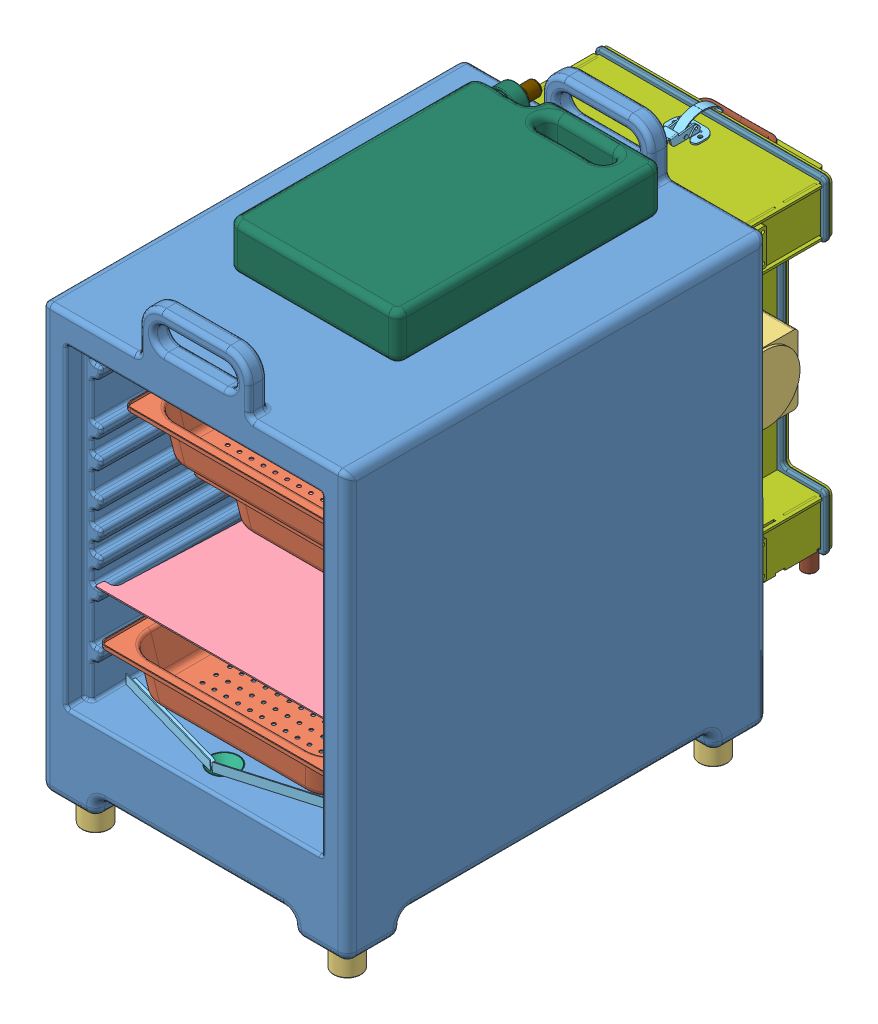
SolidWorks assembly FMT.201, configuration FULL ASSEMBLY. Lengths in mm.
Overall size (425.45 698.5 816.55).
103 component instances, 37 part files, 199 mates.
Components (placement in the parent):
- FMT.003-1: FMT.003 [Default] at origin size (425.45 660.4 584.2)
- FMT.004-1: FMT.004 [Default] at (0 188.9125 -205.3413) x (0 0 -1) z (1 0 0) size (352.43 61.91 323.85)
- FMT.004-2: FMT.004 [Default] at (0 457.2 -240.4686) x (0 0 -1) z (1 0 0) size (352.43 61.91 323.85)
- FMT.004-3: FMT.004 [Default] at (0 333.375 -332.9533) x (0 0 -1) z (1 0 0) size (352.43 61.91 323.85)
- 9540K743 Rubber Bumper with Unthreaded Hole-1: 9540K743 Rubber Bumper with Unthreaded Hole [Default] at (174.625 0 -546.1) x (-0.837169 0 -0.546944) z (-0.546944 0 0.837169) size (38.1 38.1 38.1)
- 9540K743 Rubber Bumper with Unthreaded Hole-2: 9540K743 Rubber Bumper with Unthreaded Hole [Default] at (-174.625 0 -546.1) x (-0.837169 0 -0.546944) z (-0.546944 0 0.837169) size (38.1 38.1 38.1)
- 9540K743 Rubber Bumper with Unthreaded Hole-3: 9540K743 Rubber Bumper with Unthreaded Hole [Default] at (174.625 0 -38.1) x (-0.837169 0 -0.546944) z (-0.546944 0 0.837169) size (38.1 38.1 38.1)
- 9540K743 Rubber Bumper with Unthreaded Hole-4: 9540K743 Rubber Bumper with Unthreaded Hole [Default] at (-174.625 0 -38.1) x (-0.837169 0 -0.546944) z (-0.546944 0 0.837169) size (38.1 38.1 38.1)
- FMT.008-1: FMT.008 [Default] at (0 524.3716 -59.6438) x (1 0 0) z (0 -0.039103 -0.999235) size (323.85 16 381)
- FMT.008-2: FMT.008 [Default] at (0 367.2091 -522.2121) x (-1 0 0) z (0 -0.039103 0.999235) size (323.85 16 381)
- FMT.008-3: FMT.008 [Default] at (0 257.7083 -24.2781) x (1 0 0) z (0 -0.041994 -0.999118) size (323.85 16 381)
- 1755K11 Clear Polycarbonate 90 Degree Angle-1: 1755K11 Clear Polycarbonate 90 Degree Angle [RIGHT] at (1.3565 116.5175 -24.0575) x (-0.267235 0.025225 -0.963301) z (0.963631 0.006995 -0.267144) size (12.7 12.7 171.45)
- 1755K11 Clear Polycarbonate 90 Degree Angle-2: 1755K11 Clear Polycarbonate 90 Degree Angle [LEFT] at (-166.5711 117.7168 -69.8593) x (0.267235 0.025225 -0.963301) z (0.963631 -0.006995 0.267144) size (12.7 12.7 171.45)
- 1479T83 Plastic Funnel-1: 1479T83 Plastic Funnel [Default] at (0 116.9717 -41.4022) x (1 0 0) z (0 -0.026177 0.999657) size (41.06 50.69 41.06)
- FMT.101-1: FMT.101 [Default] at (0 335.28 -596.6968) x (-1 0 0) z (0 0 -1) size (320.04 454.66 222.83)
- 9602K410_CORROSION-RESISTANT EQUIPMENT-COOLING FAN-1: 9602K410_CORROSION-RESISTANT EQUIPMENT-COOLING FAN [Default] at (-0.0145 289.8918 -660.2113) x (-1 0 0) z (0 -1 0) size (120 120 38)
- 92949A148_18-8 SS BUTTON-HEAD SOCKET CAP SCREW-1: 92949A148_18-8 SS BUTTON-HEAD SOCKET CAP SCREW [92949A148] at (52.4855 259.746 -712.7113) x (0.019534 0 -0.999809) z (0 1 0) size (6.65 6.65 14.96)
- 92949A148_18-8 SS BUTTON-HEAD SOCKET CAP SCREW-2: 92949A148_18-8 SS BUTTON-HEAD SOCKET CAP SCREW [92949A148] at (52.4855 259.746 -607.6823) x (0.019534 0 -0.999809) z (0 1 0) size (6.65 6.65 14.96)
- 92949A148_18-8 SS BUTTON-HEAD SOCKET CAP SCREW-3: 92949A148_18-8 SS BUTTON-HEAD SOCKET CAP SCREW [92949A148] at (-52.5435 259.746 -712.7113) x (0.019534 0 -0.999809) z (0 1 0) size (6.65 6.65 14.96)
- 92949A148_18-8 SS BUTTON-HEAD SOCKET CAP SCREW-4: 92949A148_18-8 SS BUTTON-HEAD SOCKET CAP SCREW [92949A148] at (-52.5435 259.746 -607.6823) x (0.019534 0 -0.999809) z (0 1 0) size (6.65 6.65 14.96)
- FMT.202-1: FMT.202 [Default] at (0 58.42 -584.2) x (-1 0 0) z (0 0 -1) size (304.8 50.8 24)
- 1661A100_LOAD-RATED PULL HANDLE WITH THREADED HOLES-1: 1661A100_LOAD-RATED PULL HANDLE WITH THREADED HOLES [1661A1] at (0 147.32 -726.6686) x (1 0 0) z (0 0 -1) size (120.8 23.9 38.64)
- 1661A100_LOAD-RATED PULL HANDLE WITH THREADED HOLES-2: 1661A100_LOAD-RATED PULL HANDLE WITH THREADED HOLES [1661A1] at (0 523.24 -726.6686) x (1 0 0) z (0 0 -1) size (120.8 23.9 38.64)
- 92949A537_18-8 SS BUTTON-HEAD SOCKET CAP SCREW-1: 92949A537_18-8 SS BUTTON-HEAD SOCKET CAP SCREW [92949A537] at (-52.3875 147.32 -720.344) x (0.730716 0.682681 0) z (0 0 1) size (11.1 11.1 16.71)
- 92949A537_18-8 SS BUTTON-HEAD SOCKET CAP SCREW-2: 92949A537_18-8 SS BUTTON-HEAD SOCKET CAP SCREW [92949A537] at (52.3875 147.32 -720.344) x (0.730716 0.682681 0) z (0 0 1) size (11.1 11.1 16.71)
- 92949A537_18-8 SS BUTTON-HEAD SOCKET CAP SCREW-3: 92949A537_18-8 SS BUTTON-HEAD SOCKET CAP SCREW [92949A537] at (-52.3875 523.24 -720.344) x (0.730716 0.682681 0) z (0 0 1) size (11.1 11.1 16.71)
- 92949A537_18-8 SS BUTTON-HEAD SOCKET CAP SCREW-4: 92949A537_18-8 SS BUTTON-HEAD SOCKET CAP SCREW [92949A537] at (52.3875 523.24 -720.344) x (0.730716 0.682681 0) z (0 0 1) size (11.1 11.1 16.71)
- 91830A101_18-8 STAINLESS STEEL KNURLED HEAD THUMB SCREW-1: 91830A101_18-8 STAINLESS STEEL KNURLED HEAD THUMB SCREW [91830A101] at (142.875 523.24 -726.6686) x (-0.923728 -0.383049 0) z (0 0 -1) size (9.52 9.52 12.12)
- 91830A101_18-8 STAINLESS STEEL KNURLED HEAD THUMB SCREW-2: 91830A101_18-8 STAINLESS STEEL KNURLED HEAD THUMB SCREW [91830A101] at (-142.875 523.24 -726.6686) x (-0.923728 -0.383049 0) z (0 0 -1) size (9.52 9.52 12.12)
- 91830A101_18-8 STAINLESS STEEL KNURLED HEAD THUMB SCREW-3: 91830A101_18-8 STAINLESS STEEL KNURLED HEAD THUMB SCREW [91830A101] at (142.875 147.32 -726.6686) x (-0.923728 0.383049 0) z (0 0 -1) size (9.52 9.52 12.12)
- 91830A101_18-8 STAINLESS STEEL KNURLED HEAD THUMB SCREW-4: 91830A101_18-8 STAINLESS STEEL KNURLED HEAD THUMB SCREW [91830A101] at (-142.875 147.32 -726.6686) x (-0.923728 0.383049 0) z (0 0 -1) size (9.52 9.52 12.12)
- 91830A101_18-8 STAINLESS STEEL KNURLED HEAD THUMB SCREW-5: 91830A101_18-8 STAINLESS STEEL KNURLED HEAD THUMB SCREW [91830A101] at (85.725 436.88 -726.6686) x (-0.923728 -0.383049 0) z (0 0 -1) size (9.52 9.52 12.12)
- 91780A560_ALUM FEM THRDED HEX STANDOFF-1: 91780A560_ALUM FEM THRDED HEX STANDOFF [91780A560] at (142.875 523.24 -660.1968) size (6.35 7.33 127.86)
- 91780A560_ALUM FEM THRDED HEX STANDOFF-4: 91780A560_ALUM FEM THRDED HEX STANDOFF [91780A560] at (142.875 147.32 -660.1968) size (6.35 7.33 127.86)
- 91780A560_ALUM FEM THRDED HEX STANDOFF-2: 91780A560_ALUM FEM THRDED HEX STANDOFF [91780A560] at (-142.875 523.24 -660.1968) size (6.35 7.33 127.86)
- 91780A560_ALUM FEM THRDED HEX STANDOFF-3: 91780A560_ALUM FEM THRDED HEX STANDOFF [91780A560] at (-142.875 147.32 -660.1968) size (6.35 7.33 127.86)
- 91780A560_ALUM FEM THRDED HEX STANDOFF-5: 91780A560_ALUM FEM THRDED HEX STANDOFF [91780A560] at (85.725 436.88 -660.1968) size (6.35 7.33 127.86)
- 91780A560_ALUM FEM THRDED HEX STANDOFF-6: 91780A560_ALUM FEM THRDED HEX STANDOFF [91780A560] at (-85.725 436.88 -660.1968) size (6.35 7.33 127.86)
- 91830A101_18-8 STAINLESS STEEL KNURLED HEAD THUMB SCREW-6: 91830A101_18-8 STAINLESS STEEL KNURLED HEAD THUMB SCREW [91830A101] at (-85.725 436.88 -726.6686) x (-0.923728 -0.383049 0) z (0 0 -1) size (9.52 9.52 12.12)
- Heating Element-1: Heating Element [Default] at (-2.4765 289.8918 -660.3873) x (0 0 1) z (0 1 0) size (119.38 122.68 24.13)
- 91830A101_18-8 STAINLESS STEEL KNURLED HEAD THUMB SCREW-7: 91830A101_18-8 STAINLESS STEEL KNURLED HEAD THUMB SCREW [91830A101] at (85.725 233.68 -726.6686) x (-0.923728 0.383049 0) z (0 0 -1) size (9.52 9.52 12.12)
- 91830A101_18-8 STAINLESS STEEL KNURLED HEAD THUMB SCREW-8: 91830A101_18-8 STAINLESS STEEL KNURLED HEAD THUMB SCREW [91830A101] at (-85.725 233.68 -726.6686) x (-0.923728 0.383049 0) z (0 0 -1) size (9.52 9.52 12.12)
- 91780A560_ALUM FEM THRDED HEX STANDOFF-7: 91780A560_ALUM FEM THRDED HEX STANDOFF [91780A560] at (-85.725 233.68 -660.1968) size (6.35 7.33 127.86)
- 91780A560_ALUM FEM THRDED HEX STANDOFF-8: 91780A560_ALUM FEM THRDED HEX STANDOFF [91780A560] at (85.725 233.68 -660.1968) size (6.35 7.33 127.86)
- 4946A100_EXPANDABLE LOCKING GROMMETS-1: 4946A100_EXPANDABLE LOCKING GROMMETS [4946A1] at (-92.5512 283.6418 -660.1968) x (0 0.984877 -0.173256) z (0 -0.173256 -0.984877) size (16.67 6.35 16.67)
- 4946A100_EXPANDABLE LOCKING GROMMETS-2: 4946A100_EXPANDABLE LOCKING GROMMETS [4946A1] at (-92.5512 309.0418 -660.1968) x (0 -1 0) z (0 0 1) size (16.67 6.35 16.67)
- MCM 4629T35-1: MCM 4629T35 [Default] at (-57.15 50.8 -318.135) x (0 0 -1) z (-1 0 0) size (330.2 66.71 213.41)
- 1601N123-1: 1601N123 [Default] at (0 523.24 -593.725) size (304.8 76.2 9.53)
- 1601N123-2: 1601N123 [Default] at (0 147.32 -593.725) size (304.8 76.2 9.53)
- MCM 1659A7-1: MCM 1659A7 [FEMALE] at (-166.6875 523.24 -608.1268) x (0 1 0) z (0 0 1) size (46.61 12.7 31.75)
- MCM 1659A7-2: MCM 1659A7 [MALE] at (-168.5925 523.24 -622.3) x (0 1 0) z (0 0 1) size (46.61 12.7 31.75)
- FMT.203-2: FMT.203 [Default] at (-153.3525 711.581 -744.22) x (0 0 -1) z (-1 0 0) size (6.35 50.8 38.1)
- FMT.203-3: FMT.203 [Default] at (-153.3525 335.661 -744.22) x (0 0 -1) z (-1 0 0) size (6.35 50.8 38.1)
- MCM 1659A7-3: MCM 1659A7 [MALE] at (-168.5925 147.32 -622.3) x (0 1 0) z (0 0 1) size (46.61 12.7 31.75)
- MCM 1659A7-4: MCM 1659A7 [FEMALE] at (-166.6875 147.32 -608.1268) x (0 1 0) z (0 0 1) size (46.61 12.7 31.75)
- MCM 1659A7-5: MCM 1659A7 [MALE] at (168.5925 523.24 -622.3) x (0 -1 0) z (0 0 1) size (46.61 12.7 31.75)
- MCM 1659A7-6: MCM 1659A7 [FEMALE] at (166.6875 523.24 -608.1268) x (0 -1 0) z (0 0 1) size (46.61 12.7 31.75)
- MCM 1659A7-7: MCM 1659A7 [MALE] at (168.5925 147.32 -622.3) x (0 -1 0) z (0 0 1) size (46.61 12.7 31.75)
- MCM 1659A7-8: MCM 1659A7 [FEMALE] at (166.6875 147.32 -608.1268) x (0 -1 0) z (0 0 1) size (46.61 12.7 31.75)
- GeekTeches Thermoelectric Peltier Refrigeration Cooling System, Radiator Semiconductor Cooler Conduction Module Fan-1: GeekTeches Thermoelectric Peltier Refrigeration Cooling System, Radiator Semiconductor Cooler Conduction Module Fan [Default] at (144.145 339.5218 -646.2268) x (0 0 1) z (-1 0 0) size (96.52 96.52 96.52)
- FMT.011-1: FMT.011 [simplified mesh] at (0 477.3418 -686.4169) size (154.94 103.94 79.25)
- FMT.203-4: FMT.203 [Default] at (153.4556 335.661 -744.22) x (0 0 -1) z (1 0 0) size (6.35 50.8 38.1)
- FMT.203-5: FMT.203 [Default] at (153.4556 -40.259 -744.22) x (0 0 -1) z (1 0 0) size (6.35 50.8 38.1)
- 4946A100_EXPANDABLE LOCKING GROMMETS-3: 4946A100_EXPANDABLE LOCKING GROMMETS [4946A1] at (92.5512 283.6418 -660.1968) x (0 0 1) z (0 -1 0) size (16.67 6.35 16.67)
- 1863A210_DRAW LATCH-1: 1863A210_DRAW LATCH [Default] at (-0.0131 114.3 -684.9132) x (1 0 0) z (0 0 -1) size (47.62 20.89 96.69)
- 91115A834_18-8 SS FEM THRDED HEX STANDOFF-1: 91115A834_18-8 SS FEM THRDED HEX STANDOFF [91115A834] at (63.5 372.77 -685.5968) x (0.866025 -0.5 0) z (0 0 1) size (6.35 7.33 77.29)
- 92949A148_18-8 SS BUTTON-HEAD SOCKET CAP SCREW-5: 92949A148_18-8 SS BUTTON-HEAD SOCKET CAP SCREW [92949A148] at (63.5 372.77 -728.5228) x (-0.40102 0.916069 0) z (0 0 -1) size (6.65 6.65 14.96)
- 91115A834_18-8 SS FEM THRDED HEX STANDOFF-2: 91115A834_18-8 SS FEM THRDED HEX STANDOFF [91115A834] at (-63.5 372.77 -685.5968) x (0.866025 -0.5 0) z (0 0 1) size (6.35 7.33 77.29)
- 91115A834_18-8 SS FEM THRDED HEX STANDOFF-3: 91115A834_18-8 SS FEM THRDED HEX STANDOFF [91115A834] at (0 372.77 -685.5968) x (0 -1 0) z (0 0 1) size (6.35 7.33 77.29)
- 92949A148_18-8 SS BUTTON-HEAD SOCKET CAP SCREW-6: 92949A148_18-8 SS BUTTON-HEAD SOCKET CAP SCREW [92949A148] at (0 372.77 -728.5228) x (-0.40102 0.916069 0) z (0 0 -1) size (6.65 6.65 14.96)
- 92949A148_18-8 SS BUTTON-HEAD SOCKET CAP SCREW-7: 92949A148_18-8 SS BUTTON-HEAD SOCKET CAP SCREW [92949A148] at (-63.5 372.77 -728.5228) x (0.270829 0.962628 0) z (0 0 -1) size (6.65 6.65 14.96)
- FMT.204-1: FMT.204 [Default] at (0.7958 326.6119 -867.9228) size (152.7 2.97 76.7)
- FITNATE Mist Maker-1: FITNATE Mist Maker [Default] at (0.0034 328.1168 -786.3887) size (44.45 42.67 44.45)
- FITNATE Mist Maker-2: FITNATE Mist Maker [Default] at (57.1534 328.1168 -786.3887) size (44.45 42.67 44.45)
- FMT.205-1: FMT.205 [Default] at (-0.7958 313.9119 -504.9109) x (-1 0 0) z (0 0 -1) size (130 6.35 60)
- 91115A135_18-8 SS FEM THRDED HEX STANDOFF-1: 91115A135_18-8 SS FEM THRDED HEX STANDOFF [91115A135] at (50 439.1338 -686.4169) x (1 0 0) z (0 1 0) size (6.35 7.33 39.19)
- 91115A135_18-8 SS FEM THRDED HEX STANDOFF-2: 91115A135_18-8 SS FEM THRDED HEX STANDOFF [91115A135] at (-50 439.1338 -686.4169) x (1 0 0) z (0 1 0) size (6.35 7.33 39.19)
- 1661A100_LOAD-RATED PULL HANDLE WITH THREADED HOLES-3: 1661A100_LOAD-RATED PULL HANDLE WITH THREADED HOLES [1661A1] at (0 441.3418 -726.0409) x (1 0 0) z (0 0 -1) size (120.8 23.9 38.64)
- 92949A537_18-8 SS BUTTON-HEAD SOCKET CAP SCREW-5: 92949A537_18-8 SS BUTTON-HEAD SOCKET CAP SCREW [92949A537] at (-52.3875 441.3418 -721.4181) x (0.730716 0.682681 0) z (0 0 1) size (11.1 11.1 16.71)
- 92949A537_18-8 SS BUTTON-HEAD SOCKET CAP SCREW-6: 92949A537_18-8 SS BUTTON-HEAD SOCKET CAP SCREW [92949A537] at (52.3875 441.3418 -721.4181) x (0.730716 0.682681 0) z (0 0 1) size (11.1 11.1 16.71)
- 1863A210_DRAW LATCH-2: 1863A210_DRAW LATCH [Default] at (0.0131 556.26 -684.9132) x (-1 0 0) z (0 0 -1) size (47.62 20.89 96.69)
- 9540K731 Rubber Bumper with Unthreaded Hole-1: 9540K731 Rubber Bumper with Unthreaded Hole [Default] at (142.875 114.3 -710.9968) x (-0.837169 0 -0.546944) z (-0.546944 0 0.837169) size (19.05 25.4 19.05)
- 9540K731 Rubber Bumper with Unthreaded Hole-2: 9540K731 Rubber Bumper with Unthreaded Hole [Default] at (-142.875 114.3 -710.9968) x (-0.837169 0 -0.546944) z (-0.546944 0 0.837169) size (19.05 25.4 19.05)
- 9540K731 Rubber Bumper with Unthreaded Hole-3: 9540K731 Rubber Bumper with Unthreaded Hole [Default] at (142.875 114.3 -619.125) x (-0.837169 0 -0.546944) z (-0.546944 0 0.837169) size (19.05 25.4 19.05)
- 9540K731 Rubber Bumper with Unthreaded Hole-4: 9540K731 Rubber Bumper with Unthreaded Hole [Default] at (-142.875 114.3 -619.125) x (-0.826006 0 -0.563662) z (-0.563662 0 0.826006) size (19.05 25.4 19.05)
- 92949A153_18-8 SS BUTTON-HEAD SOCKET CAP SCREW-1: 92949A153_18-8 SS BUTTON-HEAD SOCKET CAP SCREW [92949A153] at (-142.875 93.3958 -710.9968) x (-0.837051 0 -0.547124) z (0 -1 0) size (6.65 6.65 27.74)
- 92949A153_18-8 SS BUTTON-HEAD SOCKET CAP SCREW-2: 92949A153_18-8 SS BUTTON-HEAD SOCKET CAP SCREW [92949A153] at (-142.875 93.3958 -619.125) x (-0.837169 0 -0.546944) z (0 -1 0) size (6.65 6.65 27.74)
- 92949A153_18-8 SS BUTTON-HEAD SOCKET CAP SCREW-3: 92949A153_18-8 SS BUTTON-HEAD SOCKET CAP SCREW [92949A153] at (142.875 93.3958 -619.125) x (-0.837169 0 -0.546944) z (0 -1 0) size (6.65 6.65 27.74)
- 92949A153_18-8 SS BUTTON-HEAD SOCKET CAP SCREW-4: 92949A153_18-8 SS BUTTON-HEAD SOCKET CAP SCREW [92949A153] at (142.875 93.3958 -710.9968) x (-0.837169 0 -0.546944) z (0 -1 0) size (6.65 6.65 27.74)
- 91841A007_TYPE 18-8 STAINLESS STEEL HEX NUT-1: 91841A007_TYPE 18-8 STAINLESS STEEL HEX NUT [91841A007] at (-142.875 118.6609 -710.9968) size (7.94 3.39 9.17)
- 91841A007_TYPE 18-8 STAINLESS STEEL HEX NUT-2: 91841A007_TYPE 18-8 STAINLESS STEEL HEX NUT [91841A007] at (142.875 118.6609 -619.125) size (7.94 3.39 9.17)
- 91841A007_TYPE 18-8 STAINLESS STEEL HEX NUT-3: 91841A007_TYPE 18-8 STAINLESS STEEL HEX NUT [91841A007] at (142.875 118.6609 -710.9968) size (7.94 3.39 9.17)
- 91841A007_TYPE 18-8 STAINLESS STEEL HEX NUT-4: 91841A007_TYPE 18-8 STAINLESS STEEL HEX NUT [91841A007] at (-142.875 118.6609 -619.125) size (7.94 3.39 9.17)
- 93085K11 Surface-Mount, Hollow, 375 Wide, 1875 ID Rubber Seal-1: 93085K11 Surface-Mount, Hollow, 375 Wide, 1875 ID Rubber Seal [Default] at (0 335.28 -843.0768) size (320.04 454.66 7.62)
- 1542N2 HDPE TANK-1: 1542N2 HDPE TANK [Default] at (0 590.55 -349.25) size (235.88 63.5 373.38)
- 5779K162_PUSH-TO-CONNECT TUBE FITTING FOR AIR-1: 5779K162_PUSH-TO-CONNECT TUBE FITTING FOR AIR [5779K162] at (-59.47 465.3418 -734.9766) x (-1 0 0) z (0 0 -1) size (22.1 46.6 41.62)
- 5779K455_PUSH-TO-CONNECT TUBE FITTING FOR AIR-1: 5779K455_PUSH-TO-CONNECT TUBE FITTING FOR AIR [5779K455] at (-59.47 465.3418 -726.0409) x (-0.866025 -0.5 0) z (0 0 1) size (22.1 46.53 45.42)
- 5779K119_PUSH-TO-CONNECT TUBE FITTING FOR AIR-1: 5779K119_PUSH-TO-CONNECT TUBE FITTING FOR AIR [5779K119] at (-92.075 622.3 -528.2743) x (-0.079078 -0.996868 0) z (0 0 1) size (22 25.4 38.57)
- 50785K142_MED-PRESSURE BRASS THREADED PIPE FITTING-1: 50785K142_MED-PRESSURE BRASS THREADED PIPE FITTING [50785K142] at (-92.075 622.3 -533.4) x (0.619078 -0.78533 0) z (0 0 1) size (22.23 25.66 5.49)
- 92949A148_18-8 SS BUTTON-HEAD SOCKET CAP SCREW-8: 92949A148_18-8 SS BUTTON-HEAD SOCKET CAP SCREW [92949A148] at (50 466.3881 -686.4169) x (1 0 0) z (0 1 0) size (6.65 6.65 14.96)
- 92949A148_18-8 SS BUTTON-HEAD SOCKET CAP SCREW-9: 92949A148_18-8 SS BUTTON-HEAD SOCKET CAP SCREW [92949A148] at (-50 466.3881 -686.4169) x (1 0 0) z (0 1 0) size (6.65 6.65 14.96)
- 92949A148_18-8 SS BUTTON-HEAD SOCKET CAP SCREW-10: 92949A148_18-8 SS BUTTON-HEAD SOCKET CAP SCREW [92949A148] at (50 415.2578 -686.4169) x (-0.837169 0 -0.546944) z (0 -1 0) size (6.65 6.65 14.96)
- 92949A148_18-8 SS BUTTON-HEAD SOCKET CAP SCREW-11: 92949A148_18-8 SS BUTTON-HEAD SOCKET CAP SCREW [92949A148] at (-50 415.2578 -686.4169) x (-0.837169 0 -0.546944) z (0 -1 0) size (6.65 6.65 14.96)
Mates (geometry in assembly coordinates):
- Coincident1: coincident: plane of FMT.003-1 through (-212.725 0 -584.2) normal (0 -1 0); plane of assembly through (0 0 0) normal (0 1 0)
- Coincident2: coincident: plane of FMT.003-1 through (0 0 0) normal (1 0 0); plane of assembly through (0 0 0) normal (1 0 0)
- Coincident3: coincident: plane of FMT.003-1 through (0 0 0) normal (0 0 1); plane of assembly through (0 0 0) normal (0 0 1)
- Width4: width: plane of FMT.004-1 through (161.925 184.15 -29.1288) normal (1 0 0); plane of FMT.004-1 through (-161.925 184.15 -29.1288) normal (-1 0 0); plane of FMT.003-1 through (-167.4812 0 -25.4) normal (0.999962 0 0.008727); plane of FMT.003-1 through (167.4812 0 -25.4) normal (-0.999962 0 0.008727)
- Width5: width: plane of FMT.004-2 through (-161.925 452.4375 -64.2561) normal (-1 0 0); plane of FMT.004-2 through (161.925 452.4375 -64.2561) normal (1 0 0); plane of FMT.003-1 through (-167.4812 0 -25.4) normal (0.999962 0 0.008727); plane of FMT.003-1 through (167.4812 0 -25.4) normal (-0.999962 0 0.008727)
- Width6: width: plane of FMT.004-3 through (-161.925 328.6125 -156.7408) normal (-1 0 0); plane of FMT.004-3 through (161.925 328.6125 -156.7408) normal (1 0 0); plane of FMT.003-1 through (-167.4812 0 -25.4) normal (0.999962 0 0.008727); plane of FMT.003-1 through (167.4812 0 -25.4) normal (-0.999962 0 0.008727)
- Coincident12: coincident: plane of FMT.003-1 through (-167.4812 184.15 -572.1703) normal (0 1 0); plane of FMT.004-1 through (0 184.15 -205.3413) normal (0 -1 0)
- Coincident13: coincident: plane of FMT.003-1 through (-154.7812 328.6125 -572.1703) normal (0 1 0); plane of FMT.004-3 through (0 328.6125 -332.9533) normal (0 -1 0)
- Coincident14: coincident: plane of FMT.003-1 through (-167.4812 452.4375 -572.1703) normal (0 1 0); plane of FMT.004-2 through (0 452.4375 -240.4686) normal (0 -1 0)
- Coincident34: coincident: plane of FMT.003-1 through (-212.725 0 -584.2) normal (0 -1 0); plane of 9540K743 Rubber Bumper with Unthreaded Hole-1 through (174.625 0 -546.1) normal (0 1 0)
- Concentric4: concentric: cylinder of FMT.003-1 through (174.625 12.7 -546.1) axis (0 -1 0) radius 1.5875; cylinder of 9540K743 Rubber Bumper with Unthreaded Hole-1 through (174.625 -31.75 -546.1) axis (0 -1 0) radius 6.35
- Coincident35: coincident: plane of FMT.003-1 through (-212.725 0 -584.2) normal (0 -1 0); plane of 9540K743 Rubber Bumper with Unthreaded Hole-2 through (-174.625 0 -546.1) normal (0 1 0)
- Coincident36: coincident: plane of FMT.003-1 through (-212.725 0 -584.2) normal (0 -1 0); plane of 9540K743 Rubber Bumper with Unthreaded Hole-3 through (174.625 0 -38.1) normal (0 1 0)
- Coincident37: coincident: plane of FMT.003-1 through (-212.725 0 -584.2) normal (0 -1 0); plane of 9540K743 Rubber Bumper with Unthreaded Hole-4 through (-174.625 0 -38.1) normal (0 1 0)
- Concentric5: concentric: cylinder of FMT.003-1 through (-174.625 12.7 -546.1) axis (0 -1 0) radius 1.5875; cylinder of 9540K743 Rubber Bumper with Unthreaded Hole-2 through (-174.625 -38.1 -546.1) axis (0 1 0) radius 19.05
- Concentric6: concentric: cylinder of FMT.003-1 through (174.625 12.7 -38.1) axis (0 -1 0) radius 1.5875; cylinder of 9540K743 Rubber Bumper with Unthreaded Hole-3 through (174.625 -38.1 -38.1) axis (0 1 0) radius 19.05
- Concentric7: concentric: cylinder of FMT.003-1 through (-174.625 12.7 -38.1) axis (0 -1 0) radius 1.5875; cylinder of 9540K743 Rubber Bumper with Unthreaded Hole-4 through (-174.625 -38.1 -38.1) axis (0 1 0) radius 19.05
- Width17: width: plane of FMT.008-1 through (-146.05 518.7571 -243.715) normal (-1 0 0); plane of FMT.008-1 through (146.05 517.1709 -243.653) normal (1 0 0); plane of FMT.003-1 through (-212.725 590.55 -584.2) normal (-1 0 0); plane of FMT.003-1 through (212.725 590.55 -584.2) normal (1 0 0)
- Coincident43: coincident: plane of FMT.003-1 through (-167.4812 523.875 -572.1703) normal (0 1 0); line of FMT.008-1 through (-158.75 523.875 -72.3341) axis (1 0 0)
- Coincident44: coincident: plane of FMT.003-1 through (-167.4812 523.875 -572.1703) normal (0 1 0); line of FMT.008-1 through (-153.3525 523.875 -440.916) axis (-1 0 0)
- Width18: width: plane of FMT.008-2 through (-146.05 360.0084 -338.2029) normal (-1 0 0); plane of FMT.008-2 through (146.05 361.5946 -338.1409) normal (1 0 0); plane of FMT.003-1 through (212.725 590.55 -584.2) normal (1 0 0); plane of FMT.003-1 through (-212.725 590.55 -584.2) normal (-1 0 0)
- Coincident46: coincident: plane of FMT.003-1 through (-167.4812 366.7125 -572.1703) normal (0 1 0); line of FMT.008-2 through (-158.75 366.7125 -140.9399) axis (1 0 0)
- Coincident47: coincident: plane of FMT.003-1 through (-167.4812 366.7125 -572.1703) normal (0 1 0); line of FMT.008-2 through (-154.05 366.7125 -509.5218) axis (-1 0 0)
- Width19: width: plane of FMT.008-3 through (-146.05 251.5612 -208.3324) normal (-1 0 0); plane of FMT.008-3 through (146.05 249.9751 -208.2657) normal (1 0 0); plane of FMT.003-1 through (212.725 590.55 -584.2) normal (1 0 0); plane of FMT.003-1 through (-212.725 590.55 -584.2) normal (-1 0 0)
- Coincident48: coincident: plane of FMT.003-1 through (-154.7812 257.175 -572.1703) normal (0 1 0); line of FMT.008-3 through (-158.75 257.175 -380.1697) axis (1 0 0)
- Coincident49: coincident: plane of FMT.003-1 through (-154.7812 257.175 -572.1703) normal (0 1 0); line of FMT.008-3 through (-158.75 257.175 -36.9669) axis (1 0 0)
- Coincident52: coincident: plane of FMT.003-1 through (-167.4812 115.8875 0) normal (0 0.999657 0.026177); plane of 1755K11 Clear Polycarbonate 90 Degree Angle-1 through (163.1772 118.0372 -82.0932) normal (0 -0.999657 -0.026177)
- Parallel12: parallel: plane of FMT.003-1 through (167.4812 0 -25.4) normal (-0.999962 0 0.008727); line of 1755K11 Clear Polycarbonate 90 Degree Angle-1 through (163.2804 118.997 -70.2313) axis (-0.008724 0.026176 -0.999619)
- Coincident54: coincident: plane of FMT.003-1 through (-167.4812 115.8875 0) normal (0 0.999657 0.026177); plane of 1755K11 Clear Polycarbonate 90 Degree Angle-2 through (2.0374 116.8378 -36.2914) normal (0 -0.999657 -0.026177)
- Parallel13: parallel: plane of FMT.003-1 through (-167.4812 0 -25.4) normal (0.999962 0 0.008727); line of 1755K11 Clear Polycarbonate 90 Degree Angle-2 through (-163.1772 119.3068 -82.06) axis (-0.008724 -0.026176 0.999619)
- Width20: width: plane of 1755K11 Clear Polycarbonate 90 Degree Angle-1 through (1.3565 116.5175 -24.0575) normal (-0.870354 0.01289 -0.492257); plane of 1755K11 Clear Polycarbonate 90 Degree Angle-2 through (-1.3565 116.5175 -24.0575) normal (0.870354 0.01289 -0.492257); plane of FMT.003-1 through (212.725 590.55 -584.2) normal (1 0 0); plane of FMT.003-1 through (-212.725 590.55 -584.2) normal (-1 0 0)
- Coincident55: coincident: line of FMT.003-1 through (-159.1326 130.1736 -545.5647) axis (-0.008724 -0.026176 0.999619); point of 1755K11 Clear Polycarbonate 90 Degree Angle-2
- Coincident56: coincident: line of FMT.003-1 through (163.6384 116.6533 -29.2432) axis (-0.008724 0.026176 -0.999619); point of 1755K11 Clear Polycarbonate 90 Degree Angle-1
- Coincident65: coincident: plane of FMT.003-1 through (-167.4812 115.8875 0) normal (0 0.999657 0.026177); circle of 1479T83 Plastic Funnel-1
- Concentric11: concentric: cylinder of FMT.003-1 through (0 -14.1238 -44.8351) axis (0 0.999657 0.026177) radius 20.6375; cylinder of 1479T83 Plastic Funnel-1 through (0 116.9717 -41.4022) axis (0 0.999657 0.026177) radius 2.9527
- Coincident69: coincident: plane of 92949A537_18-8 SS BUTTON-HEAD SOCKET CAP SCREW-3 through (-48.5987 519.1846 -723.6968) normal (0 0 -1); plane of 92949A537_18-8 SS BUTTON-HEAD SOCKET CAP SCREW-4 through (56.1763 519.1846 -723.6968) normal (0 0 -1)
- Coincident70: coincident: plane of 92949A537_18-8 SS BUTTON-HEAD SOCKET CAP SCREW-2 through (56.1763 143.2646 -723.6968) normal (0 0 -1); plane of 92949A537_18-8 SS BUTTON-HEAD SOCKET CAP SCREW-4 through (56.1763 519.1846 -723.6968) normal (0 0 -1)
- Coincident71: coincident: plane of 92949A537_18-8 SS BUTTON-HEAD SOCKET CAP SCREW-1 through (-48.5987 143.2646 -723.6968) normal (0 0 -1); plane of 92949A537_18-8 SS BUTTON-HEAD SOCKET CAP SCREW-2 through (56.1763 143.2646 -723.6968) normal (0 0 -1)
- Distance8: distance = 9.525 mm: plane of FMT.003-1 through (0 0 -584.2) normal (0 0 -1); plane of FMT.101-1 through (0 335.28 -593.725) normal (0 0 1)
- Width32: width: plane of FMT.101-1 through (-153.67 335.28 -596.6968) normal (-1 0 0); plane of FMT.101-1 through (153.67 335.28 -596.6968) normal (1 0 0); plane of FMT.003-1 through (212.725 590.55 -584.2) normal (1 0 0); plane of FMT.003-1 through (-212.725 590.55 -584.2) normal (-1 0 0)
- Coincident96: coincident: plane of 92949A537_18-8 SS BUTTON-HEAD SOCKET CAP SCREW-1 through (-48.5987 143.2646 -723.6968) normal (0 0 -1); plane of FMT.101-1 through (-151.13 553.72 -723.6968) normal (0 0 1)
- Concentric24: concentric: circle of 92949A537_18-8 SS BUTTON-HEAD SOCKET CAP SCREW-3; circle of 1661A100_LOAD-RATED PULL HANDLE WITH THREADED HOLES-2
- Concentric25: concentric: circle of 1661A100_LOAD-RATED PULL HANDLE WITH THREADED HOLES-2; cylinder of FMT.101-1 through (-52.3875 523.24 -726.6686) axis (0 0 1) radius 3.175
- Concentric26: concentric: circle of 92949A537_18-8 SS BUTTON-HEAD SOCKET CAP SCREW-4; cylinder of FMT.101-1 through (52.3875 523.24 -726.6686) axis (0 0 1) radius 3.175
- Concentric27: concentric: circle of 92949A537_18-8 SS BUTTON-HEAD SOCKET CAP SCREW-4; circle of 1661A100_LOAD-RATED PULL HANDLE WITH THREADED HOLES-2
- Coincident98: coincident: plane of 1661A100_LOAD-RATED PULL HANDLE WITH THREADED HOLES-2 through (-46.0375 512.9212 -726.6686) normal (0 0 1); plane of FMT.101-1 through (-151.13 553.72 -726.6686) normal (0 0 -1)
- Concentric28: concentric: cylinder of 92949A537_18-8 SS BUTTON-HEAD SOCKET CAP SCREW-1 through (-52.3875 147.32 -720.344) axis (0 0 1) radius 5.5499; circle of FMT.101-1
- Concentric29: concentric: circle of 92949A537_18-8 SS BUTTON-HEAD SOCKET CAP SCREW-2; circle of FMT.101-1
- Coincident99: coincident: plane of 1661A100_LOAD-RATED PULL HANDLE WITH THREADED HOLES-1 through (46.0375 137.0012 -726.6686) normal (0 0 1); plane of FMT.101-1 through (-151.13 553.72 -726.6686) normal (0 0 -1)
- Concentric30: concentric: circle of 1661A100_LOAD-RATED PULL HANDLE WITH THREADED HOLES-1; circle of 92949A537_18-8 SS BUTTON-HEAD SOCKET CAP SCREW-1
- Concentric31: concentric: circle of 1661A100_LOAD-RATED PULL HANDLE WITH THREADED HOLES-1; circle of 92949A537_18-8 SS BUTTON-HEAD SOCKET CAP SCREW-2
- Distance9: distance = 114.3 mm: line of FMT.101-1 through (-150.6982 114.3 -609.5238) axis (0 0 -1); plane of FMT.003-1 through (-212.725 0 -584.2) normal (0 -1 0)
- Coincident100: coincident: plane of FMT.101-1 through (-151.13 553.72 -723.6968) normal (0 0 1); plane of 91780A560_ALUM FEM THRDED HEX STANDOFF-1 through (142.875 526.9062 -723.6968) normal (0 0 -1)
- Concentric32: concentric: cylinder of FMT.101-1 through (142.875 523.24 -726.6686) axis (0 0 1) radius 1.4732; circle of 91780A560_ALUM FEM THRDED HEX STANDOFF-1
- Concentric33: concentric: cylinder of FMT.101-1 through (-142.875 523.24 -726.6686) axis (0 0 1) radius 1.4732; circle of 91780A560_ALUM FEM THRDED HEX STANDOFF-2
- Coincident102: coincident: plane of FMT.101-1 through (-151.13 553.72 -723.6968) normal (0 0 1); plane of 91780A560_ALUM FEM THRDED HEX STANDOFF-2 through (-142.875 526.9062 -723.6968) normal (0 0 -1)
- Concentric35: concentric: cylinder of 9602K410_CORROSION-RESISTANT EQUIPMENT-COOLING FAN-1 through (52.4855 251.8918 -712.7113) axis (0 1 0) radius 2.25; cylinder of 92949A148_18-8 SS BUTTON-HEAD SOCKET CAP SCREW-1 through (52.4855 259.746 -712.7113) axis (0 1 0) radius 3.3274
- Concentric37: concentric: circle of FMT.101-1; cylinder of 9602K410_CORROSION-RESISTANT EQUIPMENT-COOLING FAN-1 through (-52.5145 251.8918 -712.7113) axis (0 1 0) radius 2.25
- Parallel18: parallel: plane of FMT.101-1 through (90.3232 341.757 -726.6686) normal (0 0 -1); plane of 9602K410_CORROSION-RESISTANT EQUIPMENT-COOLING FAN-1 through (-52.5145 82.1862 -720.2113) normal (0 0 -1)
- Coincident107: coincident: plane of 9602K410_CORROSION-RESISTANT EQUIPMENT-COOLING FAN-1 through (-0.0145 257.8918 -720.2113) normal (0 1 0); plane of 92949A148_18-8 SS BUTTON-HEAD SOCKET CAP SCREW-1 through (55.8123 257.8918 -712.6463) normal (0 -1 0)
- Coincident110: coincident: plane of FMT.003-1 through (0 0 -584.2) normal (0 0 -1); plane of FMT.202-1 through (152.4 109.22 -584.2) normal (0 0 1)
- Width33: width: plane of FMT.202-1 through (-152.4 102.5525 -590.8675) normal (-1 0 0); plane of FMT.202-1 through (152.4 102.5525 -590.8675) normal (1 0 0); plane of FMT.003-1 through (212.725 590.55 -584.2) normal (1 0 0); plane of FMT.003-1 through (-212.725 590.55 -584.2) normal (-1 0 0)
